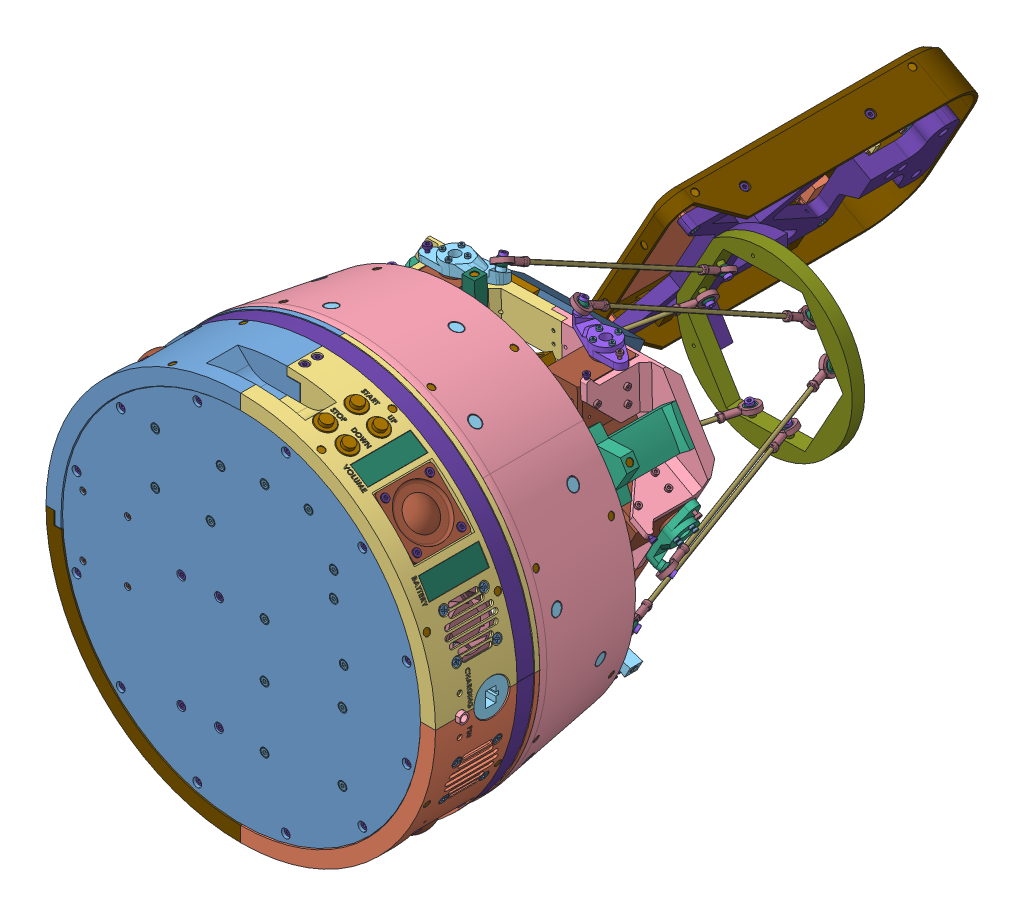
SolidWorks assembly robot xavier, configuration Défaut. Lengths in mm.
Overall size (438.41 438.41 602.06).
668 component instances, 95 part files, 20 mates.
Components (placement in the parent):
- base-1: base [Défaut] at (-67.3784 29.2661 438.4062) size (438.41 438.41 173)
  - base disk-1: base disk [Défaut] at (36.9194 20.0613 317) size (285 285 66.55)
    - base disk-1: base disk [Défaut] at (-39.9498 -9.3034 266.18) size (285 285 6.35)
    - Adafruit MAX9744-1: Adafruit MAX9744 [Défaut] at (-148.3839 -9.3034 256.18) x (0 1 0) z (0 0 -1) size (56.74 43.64 13.6)
    - Adafruit MAX9744-2: Adafruit MAX9744 [Défaut] at (-148.3839 -9.3034 239.58) x (0 1 0) z (0 0 -1) size (56.74 43.64 13.6)
    - Battery charger RRC-PMM240-1: Battery charger RRC-PMM240 [Défaut] at (-52.8471 67.1868 256.18) x (0 -1 0) z (0 0 -1) size (57 70 12)
    - battery holder-1: battery holder [Défaut] at (-92.9498 0.6966 266.18) x (0 -1 0) z (1 0 0) size (115 36.2 40)
    - Battery RRC2054-2-1: Battery RRC2054-2 [Défaut] at (-82.3791 -10.7125 233.18) x (0 1 0) z (0 0 1) size (151 78 23)
    - ground loop noise isolator-1: ground loop noise isolator [Défaut] at (-105.1098 -100.3034 233.18) x (0 -1 0) z (1 0 0) size (20 20 60)
    - ground loop noise isolator-2: ground loop noise isolator [Défaut] at (-45.1098 -80.3034 233.18) x (0 0 1) z (-1 0 0) size (20 20 60)
    - psu control-1: psu control [Défaut] at (-25.1498 95.1966 256.18) x (0 -1 0) z (0 0 -1) size (100 70 16.5)
    - buck boost-1: buck boost [Défaut] at (-25.6498 -27.3034 256.18) x (0 -1 0) z (0 0 -1) size (80 70 23.6)
    - buck boost-2: buck boost [Défaut] at (-25.6498 -27.3034 229.58) x (0 -1 0) z (0 0 -1) size (80 70 23.6)
    - 732-12936-ND-1: 732-12936-ND [Défaut] at (-166.1639 14.8266 254.58) x (-0.923728 -0.383049 0) z (0 0 -1) size (4.6 4.17 20)
    - 732-12936-ND-2: 732-12936-ND [Défaut] at (-166.1639 -33.4334 254.58) x (-0.923728 -0.383049 0) z (0 0 -1) size (4.6 4.17 20)
    - 732-12936-ND-3: 732-12936-ND [Défaut] at (-130.6039 -33.4334 254.58) x (-0.923728 -0.383049 0) z (0 0 -1) size (4.6 4.17 20)
    - 732-12936-ND-4: 732-12936-ND [Défaut] at (-130.6039 14.8266 254.58) x (-0.923728 -0.383049 0) z (0 0 -1) size (4.6 4.17 20)
    - 732-12918-ND-1: 732-12918-ND [Défaut] at (-166.1639 14.8266 266.18) x (-0.923728 -0.383049 0) z (0 0 -1) size (4.6 4.17 15)
    - 732-12918-ND-2: 732-12918-ND [Défaut] at (-130.6039 14.8266 266.18) x (-0.923728 -0.383049 0) z (0 0 -1) size (4.6 4.17 15)
    - 732-12918-ND-3: 732-12918-ND [Défaut] at (-130.6039 -33.4334 266.18) x (-0.923728 -0.383049 0) z (0 0 -1) size (4.6 4.17 15)
    - 732-12918-ND-4: 732-12918-ND [Défaut] at (-166.1639 -33.4334 266.18) x (-0.923728 -0.383049 0) z (0 0 -1) size (4.6 4.17 15)
    - M2x8mm socket-6: M2x8mm socket [Défaut] at (-166.1639 -33.4334 262.03) x (-1 0 0) z (0 0 1) size (3.8 3.8 9.6)
    - M2x8mm socket-5: M2x8mm socket [Défaut] at (-130.6039 -33.4334 262.03) x (-1 0 0) z (0 0 1) size (3.8 3.8 9.6)
    - M2x8mm socket-3: M2x8mm socket [Défaut] at (-166.1639 14.8266 262.03) size (3.8 3.8 9.6)
    - M2x8mm socket-4: M2x8mm socket [Défaut] at (-130.6039 14.8266 262.03) x (-1 0 0) z (0 0 1) size (3.8 3.8 9.6)
    - M2 nut-1: M2 nut [Défaut] at (-166.1639 14.8266 237.98) x (-0.923728 -0.383049 0) z (0 0 -1) size (4.62 4 1.6)
    - M2 nut-2: M2 nut [Défaut] at (-166.1639 -33.4334 237.98) x (-0.923728 -0.383049 0) z (0 0 -1) size (4.62 4 1.6)
    - M2 nut-3: M2 nut [Défaut] at (-130.6039 -33.4334 237.98) x (-0.923728 -0.383049 0) z (0 0 -1) size (4.62 4 1.6)
    - M2 nut-4: M2 nut [Défaut] at (-130.6039 14.8266 237.98) x (-0.923728 -0.383049 0) z (0 0 -1) size (4.62 4 1.6)
    - 36-24337-ND-1: 36-24337-ND [Défaut] at (-108.6498 86.6966 266.18) x (-0.923728 -0.383049 0) z (0 0 -1) size (5.77 5 18)
    - 36-24337-ND-2: 36-24337-ND [Défaut] at (-108.6498 45.6966 266.18) x (-0.923728 -0.383049 0) z (0 0 -1) size (5.77 5 18)
    - 36-24337-ND-3: 36-24337-ND [Défaut] at (-64.6498 44.6966 266.18) x (-0.923728 -0.383049 0) z (0 0 -1) size (5.77 5 18)
    - 36-24337-ND-4: 36-24337-ND [Défaut] at (-56.6498 86.6966 266.18) x (-0.923728 -0.383049 0) z (0 0 -1) size (5.77 5 18)
    - M3x5mm socket-1: M3x5mm socket [Défaut] at (-108.6498 86.6966 264.53) x (-1 0 0) z (0 0 1) size (5.5 5.5 8)
    - M3x5mm socket-2: M3x5mm socket [Défaut] at (-108.6498 45.6966 264.53) x (-1 0 0) z (0 0 1) size (5.5 5.5 8)
    - M3x5mm socket-3: M3x5mm socket [Défaut] at (-64.6498 44.6966 264.53) x (-1 0 0) z (0 0 1) size (5.5 5.5 8)
    - M3x5mm socket-4: M3x5mm socket [Défaut] at (-56.6498 86.6966 264.53) x (-1 0 0) z (0 0 1) size (5.5 5.5 8)
    - M3 nut-1: M3 nut [Défaut] at (-108.6498 86.6966 254.18) x (-0.923728 -0.383049 0) z (0 0 -1) size (6.35 5.5 2.4)
    - M3 nut-2: M3 nut [Défaut] at (-108.6498 45.6966 254.18) x (-0.923728 -0.383049 0) z (0 0 -1) size (6.35 5.5 2.4)
    - M3 nut-3: M3 nut [Défaut] at (-64.6498 44.6966 254.18) x (-0.923728 -0.383049 0) z (0 0 -1) size (6.35 5.5 2.4)
    - M3 nut-4: M3 nut [Défaut] at (-56.6498 86.6966 254.18) x (-0.923728 -0.383049 0) z (0 0 -1) size (6.35 5.5 2.4)
    - 36-24337-ND-5: 36-24337-ND [Défaut] at (-21.6498 91.6966 266.18) x (-0.923728 -0.383049 0) z (0 0 -1) size (5.77 5 18)
    - 36-24337-ND-6: 36-24337-ND [Défaut] at (-21.6498 -1.3034 266.18) x (1 0 0) z (0 0 -1) size (5.77 5 18)
    - 36-24337-ND-7: 36-24337-ND [Défaut] at (13.3502 91.6966 266.18) x (0.923728 0.383049 0) z (0 0 -1) size (5.77 5 18)
    - 36-24337-ND-8: 36-24337-ND [Défaut] at (41.3502 -1.3034 266.18) x (-1 0 0) z (0 0 -1) size (5.77 5 18)
    - M3 nut-5: M3 nut [Défaut] at (-21.6498 91.6966 256.98) x (-1 0 0) z (0 0 -1) size (6.35 5.5 2.4)
    - M3 nut-6: M3 nut [Défaut] at (13.3502 91.6966 252.18) x (-1 0 0) z (0 0 1) size (6.35 5.5 2.4)
    - M3 nut-7: M3 nut [Défaut] at (-21.6498 -1.3034 252.18) x (-1 0 0) z (0 0 1) size (6.35 5.5 2.4)
    - M3 nut-8: M3 nut [Défaut] at (41.3502 -1.3034 252.18) size (6.35 5.5 2.4)
    - 36-24337-ND-9: 36-24337-ND [Défaut] at (-21.6498 -44.3034 266.18) x (-0.923728 -0.383049 0) z (0 0 -1) size (5.77 5 18)
    - 36-24337-ND-10: 36-24337-ND [Défaut] at (-21.6498 -93.3034 266.18) x (-0.923728 -0.383049 0) z (0 0 -1) size (5.77 5 18)
    - 36-24337-ND-11: 36-24337-ND [Défaut] at (40.3502 -85.3034 266.18) x (-0.923728 -0.383049 0) z (0 0 -1) size (5.77 5 18)
    - 36-24337-ND-12: 36-24337-ND [Défaut] at (40.3502 -31.3034 266.18) x (-0.923728 -0.383049 0) z (0 0 -1) size (5.77 5 18)
    - 36-24342-ND-1: 36-24342-ND [Défaut] at (-21.6498 -44.3034 254.58) x (1 0 0) z (0 0 -1) size (5.77 5 33)
    - 36-24342-ND-2: 36-24342-ND [Défaut] at (-21.6498 -93.3034 254.58) x (1 0 0) z (0 0 -1) size (5.77 5 33)
    - 36-24342-ND-3: 36-24342-ND [Défaut] at (40.3502 -31.3034 254.58) x (1 0 0) z (0 0 -1) size (5.77 5 33)
    - 36-24342-ND-4: 36-24342-ND [Défaut] at (40.3502 -85.3034 254.58) x (1 0 0) z (0 0 -1) size (5.77 5 33)
    - M3 nut-9: M3 nut [Défaut] at (40.3502 -31.3034 227.98) x (-1 0 0) z (0 0 -1) size (6.35 5.5 2.4)
    - M3 nut-10: M3 nut [Défaut] at (-21.6498 -44.3034 227.98) x (-1 0 0) z (0 0 -1) size (6.35 5.5 2.4)
    - M3 nut-11: M3 nut [Défaut] at (-21.6498 -93.3034 225.58) size (6.35 5.5 2.4)
    - M3 nut-12: M3 nut [Défaut] at (40.3502 -85.3034 227.98) x (-1 0 0) z (0 0 -1) size (6.35 5.5 2.4)
    - 36-24337-ND-13: 36-24337-ND [Défaut] at (33.3502 60.1966 266.18) x (-0.923728 -0.383049 0) z (0 0 -1) size (5.77 5 18)
    - 36-24337-ND-14: 36-24337-ND [Défaut] at (33.3502 40.1966 266.18) x (-0.923728 -0.383049 0) z (0 0 -1) size (5.77 5 18)
    - M3 nut-13: M3 nut [Défaut] at (33.3502 60.1966 252.18) size (6.35 5.5 2.4)
    - M3 nut-14: M3 nut [Défaut] at (33.3502 40.1966 252.18) size (6.35 5.5 2.4)
    - M3x8mm plastic-1: M3x8mm plastic [Défaut] at (-57.9498 -4.3034 261.53) size (5.5 5.5 10.3)
    - M3x8mm plastic-2: M3x8mm plastic [Défaut] at (-57.9498 -94.3034 261.53) size (5.5 5.5 10.3)
    - M3x8mm plastic-3: M3x8mm plastic [Défaut] at (-87.9498 -94.3034 261.53) size (5.5 5.5 10.3)
    - M3x8mm plastic-4: M3x8mm plastic [Défaut] at (-87.9498 -4.3034 261.53) size (5.5 5.5 10.3)
    - M3x5mm socket-5: M3x5mm socket [Défaut] at (-21.6498 91.6966 264.53) size (5.5 5.5 8)
    - M3x5mm socket-6: M3x5mm socket [Défaut] at (13.3502 91.6966 264.53) size (5.5 5.5 8)
    - M3x5mm socket-7: M3x5mm socket [Défaut] at (33.3502 60.1966 264.53) size (5.5 5.5 8)
    - M3x5mm socket-8: M3x5mm socket [Défaut] at (33.3502 40.1966 264.53) size (5.5 5.5 8)
    - M3x5mm socket-9: M3x5mm socket [Défaut] at (-21.6498 -1.3034 264.53) size (5.5 5.5 8)
    - M3x5mm socket-10: M3x5mm socket [Défaut] at (-21.6498 -44.3034 264.53) size (5.5 5.5 8)
    - M3x5mm socket-11: M3x5mm socket [Défaut] at (-21.6498 -93.3034 264.53) size (5.5 5.5 8)
    - M3x5mm socket-12: M3x5mm socket [Défaut] at (40.3502 -85.3034 264.53) size (5.5 5.5 8)
    - M3x5mm socket-13: M3x5mm socket [Défaut] at (40.3502 -31.3034 264.53) size (5.5 5.5 8)
    - M3x5mm socket-14: M3x5mm socket [Défaut] at (41.3502 -1.3034 264.53) size (5.5 5.5 8)
  - base audio-1: base audio [Défaut] at (-77.1238 -92.9542 353.528) x (0 1 0) z (0 0 1) size (420.86 420.86 86)
    - base audio front left-1: base audio front left [Défaut] at (103.7122 -74.0934 171.652) size (155 165 86)
    - base audio front right-1: base audio front right [Défaut] at (103.7122 -74.0934 171.652) x (0 -1 0) z (0 0 1) size (165 165 86)
    - base audio back left-1: base audio back left [Défaut] at (103.7122 -74.0934 171.652) x (0 1 0) z (0 0 1) size (155 156 86)
    - base audio back right-1: base audio back right [Défaut] at (103.7122 -74.0934 171.652) x (-1 0 0) z (0 0 1) size (156 155 86)
    - SC2073-ND-1: SC2073-ND [Défaut] at (103.7122 -222.6934 217.152) x (1 0 0) z (0 -1 0) size (11.94 11.94 36.36)
    - RJ45 connector-1: RJ45 connector [Défaut] at (103.7122 -228.0934 191.652) x (1 0 0) z (0 1 0) size (27.9 27.9 35.9)
    - Micro USB B (Adafruit 4217)-1: Micro USB B (Adafruit 4217) [Défaut] at (-6.0335 -126.2291 211.652) x (-0.429101 0.903257 0) z (0 0 1) size (28 33.5 28)
    - Micro USB B nut (Adafruit 4217)-1: Micro USB B nut (Adafruit 4217) [Défaut] at (-28.6149 -136.9566 211.652) x (0.18262 -0.384415 -0.904917) z (0.903257 0.429101 0) size (30.02 30.02 8)
    - switch-1: switch [Défaut] at (-36.2542 -140.9179 186.027) x (0.429101 -0.903257 0) z (0.903257 0.429101 0) size (20.75 14.7 24.67)
    - button-1: button [Défaut] at (254.7907 -122.0257 191.152) x (0.197389 0.622151 -0.757605) z (-0.953177 0.302412 0) size (14 14 27.8)
    - button-2: button [Défaut] at (247.8231 -140.0803 191.152) x (0.179537 0.392097 -0.902234) z (-0.909218 0.416321 0) size (14 14 27.8)
    - button-3: button [Défaut] at (254.7907 -122.0257 216.152) x (0.197389 0.622151 -0.757605) z (-0.953177 0.302412 0) size (14 14 27.8)
    - button-4: button [Défaut] at (247.8231 -140.0803 216.152) x (0.179537 0.392097 -0.902234) z (-0.909218 0.416321 0) size (14 14 27.8)
    - button nut-1: button nut [Défaut] at (247.1653 -119.6064 191.152) x (0.099317 0.313039 0.944533) z (-0.953177 0.302412 0) size (16 16 5)
    - button nut-2: button nut [Défaut] at (247.1653 -119.6064 216.152) x (0.099317 0.313039 0.944533) z (-0.953177 0.302412 0) size (16 16 5)
    - button nut-3: button nut [Défaut] at (240.5494 -136.7497 216.152) x (0.182325 0.398185 0.899003) z (-0.909218 0.416321 0) size (16 16 5)
    - button nut-4: button nut [Défaut] at (240.5494 -136.7497 191.152) x (0.179537 0.392097 -0.902234) z (-0.909218 0.416321 0) size (16 16 5) (hidden)
    - Dayton Audio DMA45-8-1: Dayton Audio DMA45-8 [Défaut] at (209.7782 -180.1594 199.652) x (0.707107 0.707107 0) z (0.707107 -0.707107 0) size (46 46 32.1)
    - Dayton Audio DMA45-8-2: Dayton Audio DMA45-8 [Défaut] at (209.7782 31.9727 199.652) x (-0.707107 0.707107 0) z (0.707107 0.707107 0) size (46 46 32.1)
    - Dayton Audio DMA45-8-3: Dayton Audio DMA45-8 [Défaut] at (-2.3539 31.9727 199.652) x (-0.707107 -0.707107 0) z (-0.707107 0.707107 0) size (46 46 32.1)
    - Dayton Audio DMA45-8-4: Dayton Audio DMA45-8 [Défaut] at (-2.3539 -180.1594 199.652) x (0.707107 -0.707107 0) z (-0.707107 -0.707107 0) size (46 46 32.1)
    - LED 5mm-1: LED 5mm [Défaut] at (88.5685 -227.8494 216.652) x (-0.876134 0.086292 -0.474281) z (0.098017 0.995185 0) size (5.5 5.5 18.7)
    - LED 5mm-2: LED 5mm [Défaut] at (118.8558 -227.8494 216.652) x (-0.780695 -0.076892 -0.620163) z (-0.098017 0.995185 0) size (5.5 5.5 18.7)
    - Noctua NF-A4X20-1: Noctua NF-A4X20 [Défaut] at (61.6633 -197.158 199.652) x (0.946287 -0.323328 0) z (-0.323328 -0.946287 0) size (39.9 39.9 19.95)
    - Noctua NF-A4X20-2: Noctua NF-A4X20 [Défaut] at (145.761 -197.158 199.652) x (0.946287 0.323328 0) z (0.323328 -0.946287 0) size (39.9 39.9 19.95)
    - LED level-1: LED level [Défaut] at (232.9084 -146.5387 181.6389) x (0.524024 0.851704 0) z (0.851704 -0.524024 0) size (12 34.5 2)
    - LED level-2: LED level [Défaut] at (185.0786 -197.8654 181.6389) x (0.857177 0.515023 0) z (0.515023 -0.857177 0) size (12 34.5 2)
    - LED level diffuser-1: LED level diffuser [Défaut] at (240.4553 -143.8142 199.2629) x (0.524024 0.851704 0) z (0.851704 -0.524024 0) size (16 47.5 1.59)
    - LED level diffuser-2: LED level diffuser [Défaut] at (193.0327 -198.9193 199.2629) x (0.857177 0.515023 0) z (0.515023 -0.857177 0) size (16 47.5 1.59)
    - LED strip-1: LED strip [Défaut] at (103.7122 -74.0934 159.902) x (0.707107 -0.707107 0) z (0 0 1) size (297.3 297.88 9.5)
    - LED strip diffuser (round)-1: LED strip diffuser (round) [Défaut] at (103.7122 -74.0934 157.902) x (0.000809 -1 0) z (0 0 1) size (309.17 309.17 13.5)
    - light sensor-1: light sensor [Défaut] at (228.5122 -87.4674 238.7403) x (0 0 -1) z (1 0 0) size (7.62 10.16 4.2)
    - light sensor-2: light sensor [Défaut] at (-21.0878 -87.4674 196.0637) x (0 0 1) z (-1 0 0) size (7.62 10.16 4.2)
    - light sensor-3: light sensor [Défaut] at (29.9331 -198.7828 198.0637) x (0 0 1) z (-0.537899 -0.843009 0) size (7.62 10.16 4.2)
    - light sensor-4: light sensor [Défaut] at (109.4763 70.6739 198.0637) x (0 0 1) z (0.073377 0.997304 0) size (7.62 10.16 4.2)
    - M3x8mm plastic-1: M3x8mm plastic [Défaut] at (98.7122 69.9066 183.652) x (1 0 0) z (0 1 0) size (5.5 5.5 10.3)
    - M3x8mm plastic-2: M3x8mm plastic [Défaut] at (98.7122 69.9066 213.652) x (1 0 0) z (0 1 0) size (5.5 5.5 10.3)
    - M3x8mm plastic-3: M3x8mm plastic [Défaut] at (-40.2878 -79.0934 180.652) x (0 0 1) z (-1 0 0) size (5.5 5.5 10.3)
    - M3x8mm plastic-4: M3x8mm plastic [Défaut] at (-40.2878 -79.0934 190.652) x (0 0 1) z (-1 0 0) size (5.5 5.5 10.3)
    - M3x8mm plastic-5: M3x8mm plastic [Défaut] at (247.7122 -79.0934 180.652) x (0 0 -1) z (1 0 0) size (5.5 5.5 10.3)
    - M3x8mm plastic-6: M3x8mm plastic [Défaut] at (247.7122 -79.0934 190.652) x (0 0 -1) z (1 0 0) size (5.5 5.5 10.3)
    - M3x8mm plastic-8: M3x8mm plastic [Défaut] at (192.6308 -188.1143 181.902) x (0.5 0.5 -0.707107) z (0.707107 -0.707107 0) size (5.5 5.5 10.3)
    - M3x8mm plastic-14: M3x8mm plastic [Défaut] at (-10.3088 -163.012 181.902) x (0.5 -0.5 -0.707107) z (-0.707107 -0.707107 0) size (5.5 5.5 10.3)
    - M3x8mm plastic-13: M3x8mm plastic [Défaut] at (14.7935 39.9276 181.902) x (-0.5 -0.5 -0.707107) z (-0.707107 0.707107 0) size (5.5 5.5 10.3)
    - M3x8mm plastic-12: M3x8mm plastic [Défaut] at (217.7331 14.8253 181.902) x (-0.5 0.5 -0.707107) z (0.707107 0.707107 0) size (5.5 5.5 10.3)
    - M3x8mm plastic-9: M3x8mm plastic [Défaut] at (217.7331 -163.012 217.402) x (0.5 0.5 -0.707107) z (0.707107 -0.707107 0) size (5.5 5.5 10.3)
    - M3x8mm plastic-17: M3x8mm plastic [Défaut] at (14.7935 -188.1143 217.402) x (0.5 -0.5 -0.707107) z (-0.707107 -0.707107 0) size (5.5 5.5 10.3)
    - M3x8mm plastic-16: M3x8mm plastic [Défaut] at (-10.3088 14.8253 217.402) x (-0.5 -0.5 -0.707107) z (-0.707107 0.707107 0) size (5.5 5.5 10.3)
    - M3x8mm plastic-15: M3x8mm plastic [Défaut] at (192.6308 39.9276 217.402) x (-0.5 0.5 -0.707107) z (0.707107 0.707107 0) size (5.5 5.5 10.3)
    - M3x8mm plastic-10: M3x8mm plastic [Défaut] at (192.6308 -188.1143 217.402) x (0.5 0.5 -0.707107) z (0.707107 -0.707107 0) size (5.5 5.5 10.3)
    - M3x8mm plastic-20: M3x8mm plastic [Défaut] at (-10.3088 -163.012 217.402) x (0.5 -0.5 -0.707107) z (-0.707107 -0.707107 0) size (5.5 5.5 10.3)
    - M3x8mm plastic-19: M3x8mm plastic [Défaut] at (14.7935 39.9276 217.402) x (-0.5 -0.5 -0.707107) z (-0.707107 0.707107 0) size (5.5 5.5 10.3)
    - M3x8mm plastic-18: M3x8mm plastic [Défaut] at (217.7331 14.8253 217.402) x (-0.5 0.5 -0.707107) z (0.707107 0.707107 0) size (5.5 5.5 10.3)
    - M3x8mm plastic-11: M3x8mm plastic [Défaut] at (217.7331 -163.012 181.902) x (0.5 0.5 -0.707107) z (0.707107 -0.707107 0) size (5.5 5.5 10.3)
    - M3x8mm plastic-23: M3x8mm plastic [Défaut] at (14.7935 -188.1143 181.902) x (0.5 -0.5 -0.707107) z (-0.707107 -0.707107 0) size (5.5 5.5 10.3)
    - M3x8mm plastic-22: M3x8mm plastic [Défaut] at (-10.3088 14.8253 181.902) x (-0.5 -0.5 -0.707107) z (-0.707107 0.707107 0) size (5.5 5.5 10.3)
    - M3x8mm plastic-21: M3x8mm plastic [Défaut] at (192.6308 39.9276 181.902) x (-0.5 0.5 -0.707107) z (0.707107 0.707107 0) size (5.5 5.5 10.3)
    - fan screw-1: fan screw [Défaut] at (165.5737 -205.6586 183.652) x (0.879667 0.300565 -0.368573) z (0.323328 -0.946287 0) size (6.3 6.3 9.5)
    - fan screw-2: fan screw [Défaut] at (165.5737 -205.6586 215.652) x (0.879667 0.300565 -0.368573) z (0.323328 -0.946287 0) size (6.3 6.3 9.5)
    - fan screw-3: fan screw [Défaut] at (135.2925 -216.0051 215.652) x (-0.927498 -0.316908 -0.198283) z (0.323328 -0.946287 0) size (6.3 6.3 9.5)
    - fan screw-4: fan screw [Défaut] at (135.2925 -216.0051 183.652) x (0.879667 0.300565 -0.368573) z (0.323328 -0.946287 0) size (6.3 6.3 9.5)
    - fan screw-5: fan screw [Défaut] at (72.1318 -216.0051 183.652) x (0.879667 -0.300565 0.368573) z (-0.323328 -0.946287 0) size (6.3 6.3 9.5)
    - fan screw-6: fan screw [Défaut] at (72.1318 -216.0051 215.652) x (0.879667 -0.300565 0.368573) z (-0.323328 -0.946287 0) size (6.3 6.3 9.5)
    - fan screw-7: fan screw [Défaut] at (41.8506 -205.6586 215.652) x (0.879667 -0.300565 0.368573) z (-0.323328 -0.946287 0) size (6.3 6.3 9.5)
    - fan screw-8: fan screw [Défaut] at (41.8506 -205.6586 183.652) x (0.879667 -0.300565 0.368573) z (-0.323328 -0.946287 0) size (6.3 6.3 9.5)
    - dewel pin 0.125in 0.5in-1: dewel pin 0.125in 0.5in [Défaut] at (111.2122 -212.8434 155.652) x (0 0 1) z (-1 0 0) size (3.17 3.17 12.7)
    - dewel pin 0.125in 0.5in-2: dewel pin 0.125in 0.5in [Défaut] at (111.2122 -223.0934 228.6844) x (0 0 1) z (-1 0 0) size (3.17 3.17 12.7)
    - M2x5mm plastic-1: M2x5mm plastic [Défaut] at (233.5122 -79.5934 217.402) x (0 0.924225 0.381849) z (-1 0 0) size (3.35 3.35 6.6)
    - M2x5mm plastic-2: M2x5mm plastic [Défaut] at (-26.0878 -79.5934 217.402) x (0 0.5 -0.866025) z (1 0 0) size (3.35 3.35 6.6)
    - M2x5mm plastic-3: M2x5mm plastic [Défaut] at (20.6058 -198.7624 219.402) x (-0.826053 0.527081 -0.199554) z (0.537899 0.843009 0) size (3.35 3.35 6.6)
    - M2x5mm plastic-4: M2x5mm plastic [Défaut] at (117.696 75.0827 219.402) x (0.994616 -0.073179 0.073377) z (-0.073377 -0.997304 0) size (3.35 3.35 6.6)
  - base mic-1: base mic [Défaut] at (-78.91 184.7021 463.131) x (-0.707107 -0.707107 0) z (0.707107 -0.707107 0) size (310 92.85 310)
    - base mic-1: base mic [Défaut] at (69.3421 -41.049 176.652) size (155 90 160)
    - 8SoundsUSB Mic-1: 8SoundsUSB Mic [Défaut] at (30.5719 -34.8926 320.3049) x (0.980785 0 0.19509) z (-0.192688 0.156434 0.96871) size (25.4 23.4 21.48)
    - 8SoundsUSB Mic-2: 8SoundsUSB Mic [Défaut] at (-17.8103 6.4759 289.0854) x (0.83147 0 0.55557) z (-0.54873 0.156434 0.821233) size (25.4 23.4 21.48)
    - 8SoundsUSB Mic-3: 8SoundsUSB Mic [Défaut] at (-71.7864 6.4759 194.5283) x (0.19509 0 0.980785) z (-0.96871 0.156434 0.192688) size (25.4 23.4 21.48)
    - 8SoundsUSB Mic-4: 8SoundsUSB Mic [Défaut] at (-59.6505 -34.8926 250.8153) x (0.55557 0 0.83147) z (-0.821233 0.156434 0.54873) size (25.4 23.4 21.48)
    - 16SoundsUSB-1: 16SoundsUSB [Défaut] at (69.3421 -36.049 176.6521) x (1 0 0) z (0 -1 0) size (165.86 165.78 26.13)
    - M3x5mm plastic-1: M3x5mm plastic [Défaut] at (49.8528 -16.3964 325.89) x (-0.186611 0.963352 -0.192688) z (0.192688 -0.156434 -0.96871) size (5.5 5.5 7.3)
    - M3x5mm plastic-2: M3x5mm plastic [Défaut] at (30.2371 -16.3964 321.9882) x (-0.186611 0.963352 -0.192688) z (0.192688 -0.156434 -0.96871) size (5.5 5.5 7.3)
    - M3x5mm plastic-3: M3x5mm plastic [Défaut] at (49.3034 -34.1748 328.6517) x (-0.186611 0.963352 -0.192688) z (0.192688 -0.156434 -0.96871) size (5.5 5.5 7.3)
    - M3x5mm plastic-4: M3x5mm plastic [Défaut] at (29.6877 -34.1748 324.7499) x (-0.186611 0.963352 -0.192688) z (0.192688 -0.156434 -0.96871) size (5.5 5.5 7.3)
    - M3x5mm plastic-5: M3x5mm plastic [Défaut] at (-2.1344 24.9721 301.6238) x (-0.684341 0.480179 -0.54873) z (0.54873 -0.156434 -0.821233) size (5.5 5.5 7.3)
    - M3x5mm plastic-6: M3x5mm plastic [Défaut] at (-18.7638 24.9721 290.5124) x (-0.684341 0.480179 -0.54873) z (0.54873 -0.156434 -0.821233) size (5.5 5.5 7.3)
    - M3x5mm plastic-7: M3x5mm plastic [Défaut] at (-3.6988 7.1937 303.965) x (-0.684341 0.480179 -0.54873) z (0.54873 -0.156434 -0.821233) size (5.5 5.5 7.3)
    - M3x5mm plastic-8: M3x5mm plastic [Défaut] at (-20.3282 7.1937 292.8536) x (-0.684341 0.480179 -0.54873) z (0.54873 -0.156434 -0.821233) size (5.5 5.5 7.3)
    - M3x5mm plastic-9: M3x5mm plastic [Défaut] at (-49.9661 -16.3964 268.3981) x (-0.494502 0.284684 -0.821233) z (0.821233 -0.156434 -0.54873) size (5.5 5.5 7.3)
    - M3x5mm plastic-10: M3x5mm plastic [Défaut] at (-61.0775 -16.3964 251.7687) x (-0.494502 0.284684 -0.821233) z (0.821233 -0.156434 -0.54873) size (5.5 5.5 7.3)
    - M3x5mm plastic-11: M3x5mm plastic [Défaut] at (-63.4188 -34.1748 253.3331) x (-0.494502 0.284684 -0.821233) z (0.821233 -0.156434 -0.54873) size (5.5 5.5 7.3)
    - M3x5mm plastic-12: M3x5mm plastic [Défaut] at (-52.3074 -34.1748 269.9625) x (-0.494502 0.284684 -0.821233) z (0.821233 -0.156434 -0.54873) size (5.5 5.5 7.3)
    - M3x5mm plastic-13: M3x5mm plastic [Défaut] at (-72.3295 7.1937 215.0282) x (-0.225994 -0.876896 -0.424241) z (0.96871 -0.156434 -0.192688) size (5.5 5.5 7.3)
    - M3x5mm plastic-14: M3x5mm plastic [Défaut] at (-69.5678 24.9721 214.4788) x (-0.162376 0.187709 -0.96871) z (0.96871 -0.156434 -0.192688) size (5.5 5.5 7.3)
    - M3x5mm plastic-15: M3x5mm plastic [Défaut] at (-73.4696 24.9721 194.8631) x (-0.162376 0.187709 -0.96871) z (0.96871 -0.156434 -0.192688) size (5.5 5.5 7.3)
    - M3x5mm plastic-16: M3x5mm plastic [Défaut] at (-76.2313 7.1937 195.4125) x (-0.162376 0.187709 -0.96871) z (0.96871 -0.156434 -0.192688) size (5.5 5.5 7.3)
    - M3x8mm plastic-1: M3x8mm plastic [Défaut] at (15.9671 -42.4056 230.027) x (1 0 0) z (0 1 0) size (5.5 5.5 10.3)
    - M3x8mm plastic-2: M3x8mm plastic [Défaut] at (122.7171 -42.4056 230.027) x (1 0 0) z (0 1 0) size (5.5 5.5 10.3)
    - M3x8mm plastic-3: M3x8mm plastic [Défaut] at (15.9671 -42.4056 123.277) x (-0.837169 0 -0.546944) z (0 1 0) size (5.5 5.5 10.3)
    - M3x8mm plastic-4: M3x8mm plastic [Défaut] at (122.7171 -42.4056 123.277) x (-0.837169 0 -0.546944) z (0 1 0) size (5.5 5.5 10.3)
    - M3x5mm plastic-17: M3x5mm plastic [Défaut] at (-75.994 -16.3964 137.547) x (0.192688 0.963352 -0.186611) z (0.96871 -0.156434 0.192688) size (5.5 5.5 7.3)
    - M3x5mm plastic-18: M3x5mm plastic [Défaut] at (108.4472 -16.3964 31.3159) x (0.186611 0.963352 0.192688) z (-0.192688 -0.156434 0.96871) size (5.5 5.5 7.3)
    - M3x5mm plastic-19: M3x5mm plastic [Défaut] at (214.6783 -16.3964 215.7571) x (-0.192688 0.963352 0.186611) z (-0.96871 -0.156434 -0.192688) size (5.5 5.5 7.3)
    - M3x5mm plastic-20: M3x5mm plastic [Défaut] at (-82.6575 -34.1748 156.6133) x (0.192688 0.963352 -0.186611) z (0.96871 -0.156434 0.192688) size (5.5 5.5 7.3)
    - M3x5mm plastic-21: M3x5mm plastic [Défaut] at (89.3808 -34.1748 24.6524) x (0.186611 0.963352 0.192688) z (-0.192688 -0.156434 0.96871) size (5.5 5.5 7.3)
    - M3x5mm plastic-22: M3x5mm plastic [Défaut] at (221.3418 -34.1748 196.6907) x (-0.192688 0.963352 0.186611) z (-0.96871 -0.156434 -0.192688) size (5.5 5.5 7.3)
    - M3x5mm plastic-23: M3x5mm plastic [Défaut] at (-78.7557 -34.1748 136.9976) x (0.192688 0.963352 -0.186611) z (0.96871 -0.156434 0.192688) size (5.5 5.5 7.3)
    - M3x5mm plastic-24: M3x5mm plastic [Défaut] at (108.9965 -34.1748 28.5542) x (0.186611 0.963352 0.192688) z (-0.192688 -0.156434 0.96871) size (5.5 5.5 7.3)
    - M3x5mm plastic-25: M3x5mm plastic [Défaut] at (217.44 -34.1748 216.3064) x (-0.192688 0.963352 0.186611) z (-0.96871 -0.156434 -0.192688) size (5.5 5.5 7.3)
    - M3x5mm plastic-26: M3x5mm plastic [Défaut] at (-55.6296 24.9721 105.1755) x (0.54873 0.480179 -0.684341) z (0.821233 -0.156434 0.54873) size (5.5 5.5 7.3)
    - M3x5mm plastic-27: M3x5mm plastic [Défaut] at (140.8187 24.9721 51.6803) x (0.684341 0.480179 0.54873) z (-0.54873 -0.156434 0.821233) size (5.5 5.5 7.3)
    - M3x5mm plastic-28: M3x5mm plastic [Défaut] at (194.3139 24.9721 248.1286) x (-0.54873 0.480179 0.684341) z (-0.821233 -0.156434 -0.54873) size (5.5 5.5 7.3)
    - M3x5mm plastic-29: M3x5mm plastic [Défaut] at (-44.5182 24.9721 88.5461) x (0.54873 0.480179 -0.684341) z (0.821233 -0.156434 0.54873) size (5.5 5.5 7.3)
    - M3x5mm plastic-30: M3x5mm plastic [Défaut] at (157.4481 24.9721 62.7917) x (0.684341 0.480179 0.54873) z (-0.54873 -0.156434 0.821233) size (5.5 5.5 7.3)
    - M3x5mm plastic-31: M3x5mm plastic [Défaut] at (183.2025 24.9721 264.758) x (-0.54873 0.480179 0.684341) z (-0.821233 -0.156434 -0.54873) size (5.5 5.5 7.3)
    - M3x5mm plastic-32: M3x5mm plastic [Défaut] at (-57.9709 7.1937 103.6111) x (0.54873 0.480179 -0.684341) z (0.821233 -0.156434 0.54873) size (5.5 5.5 7.3)
    - M3x5mm plastic-33: M3x5mm plastic [Défaut] at (142.3831 7.1937 49.339) x (0.684341 0.480179 0.54873) z (-0.54873 -0.156434 0.821233) size (5.5 5.5 7.3)
    - M3x5mm plastic-34: M3x5mm plastic [Défaut] at (196.6551 7.1937 249.693) x (-0.54873 0.480179 0.684341) z (-0.821233 -0.156434 -0.54873) size (5.5 5.5 7.3)
    - M3x5mm plastic-35: M3x5mm plastic [Défaut] at (-46.8595 7.1937 86.9817) x (0.54873 0.480179 -0.684341) z (0.821233 -0.156434 0.54873) size (5.5 5.5 7.3)
    - M3x5mm plastic-36: M3x5mm plastic [Défaut] at (159.0125 7.1937 60.4504) x (0.684341 0.480179 0.54873) z (-0.54873 -0.156434 0.821233) size (5.5 5.5 7.3)
    - M3x5mm plastic-37: M3x5mm plastic [Défaut] at (185.5437 7.1937 266.3224) x (-0.54873 0.480179 0.684341) z (-0.821233 -0.156434 -0.54873) size (5.5 5.5 7.3)
    - M3x5mm plastic-38: M3x5mm plastic [Défaut] at (-22.404 -16.3964 57.3438) x (0.821233 0.284684 -0.494502) z (0.54873 -0.156434 0.821233) size (5.5 5.5 7.3)
    - M3x5mm plastic-39: M3x5mm plastic [Défaut] at (188.6504 -16.3964 84.9059) x (0.494502 0.284684 0.821233) z (-0.821233 -0.156434 0.54873) size (5.5 5.5 7.3)
    - M3x5mm plastic-40: M3x5mm plastic [Défaut] at (161.0882 -16.3964 295.9603) x (-0.821233 0.284684 0.494502) z (-0.54873 -0.156434 -0.821233) size (5.5 5.5 7.3)
    - M3x5mm plastic-41: M3x5mm plastic [Défaut] at (-5.7746 -16.3964 46.2324) x (0.821233 0.284684 -0.494502) z (0.54873 -0.156434 0.821233) size (5.5 5.5 7.3)
    - M3x5mm plastic-42: M3x5mm plastic [Défaut] at (199.7618 -16.3964 101.5353) x (0.494502 0.284684 0.821233) z (-0.821233 -0.156434 0.54873) size (5.5 5.5 7.3)
    - M3x5mm plastic-43: M3x5mm plastic [Défaut] at (144.4588 -16.3964 307.0717) x (-0.821233 0.284684 0.494502) z (-0.54873 -0.156434 -0.821233) size (5.5 5.5 7.3)
    - M3x5mm plastic-44: M3x5mm plastic [Défaut] at (-7.339 -34.1748 43.8911) x (0.821233 0.284684 -0.494502) z (0.54873 -0.156434 0.821233) size (5.5 5.5 7.3)
    - M3x5mm plastic-45: M3x5mm plastic [Défaut] at (202.103 -34.1748 99.9709) x (0.494502 0.284684 0.821233) z (-0.821233 -0.156434 0.54873) size (5.5 5.5 7.3)
    - M3x5mm plastic-46: M3x5mm plastic [Défaut] at (146.0232 -34.1748 309.4129) x (-0.821233 0.284684 0.494502) z (-0.54873 -0.156434 -0.821233) size (5.5 5.5 7.3)
    - M3x5mm plastic-47: M3x5mm plastic [Défaut] at (-23.9684 -34.1748 55.0025) x (0.821233 0.284684 -0.494502) z (0.54873 -0.156434 0.821233) size (5.5 5.5 7.3)
    - M3x5mm plastic-48: M3x5mm plastic [Défaut] at (190.9916 -34.1748 83.3415) x (0.494502 0.284684 0.821233) z (-0.821233 -0.156434 0.54873) size (5.5 5.5 7.3)
    - M3x5mm plastic-49: M3x5mm plastic [Défaut] at (162.6526 -34.1748 298.3015) x (-0.821233 0.284684 0.494502) z (-0.54873 -0.156434 -0.821233) size (5.5 5.5 7.3)
    - M3x5mm plastic-50: M3x5mm plastic [Défaut] at (30.966 7.1937 34.9804) x (0.424241 -0.876896 -0.225994) z (0.192688 -0.156434 0.96871) size (5.5 5.5 7.3)
    - M3x5mm plastic-51: M3x5mm plastic [Défaut] at (211.0138 7.1937 138.2759) x (0.225994 -0.876896 0.424241) z (-0.96871 -0.156434 0.192688) size (5.5 5.5 7.3)
    - M3x5mm plastic-52: M3x5mm plastic [Défaut] at (107.7183 7.1937 318.3237) x (-0.424241 -0.876896 0.225994) z (-0.192688 -0.156434 -0.96871) size (5.5 5.5 7.3)
    - M3x5mm plastic-53: M3x5mm plastic [Défaut] at (31.5153 24.9721 37.7421) x (0.96871 0.187709 -0.162376) z (0.192688 -0.156434 0.96871) size (5.5 5.5 7.3)
    - M3x5mm plastic-54: M3x5mm plastic [Défaut] at (208.252 24.9721 138.8252) x (0.162376 0.187709 0.96871) z (-0.96871 -0.156434 0.192688) size (5.5 5.5 7.3)
    - M3x5mm plastic-55: M3x5mm plastic [Défaut] at (107.1689 24.9721 315.5619) x (-0.96871 0.187709 0.162376) z (-0.192688 -0.156434 -0.96871) size (5.5 5.5 7.3)
    - M3x5mm plastic-56: M3x5mm plastic [Défaut] at (51.131 24.9721 33.8403) x (0.96871 0.187709 -0.162376) z (0.192688 -0.156434 0.96871) size (5.5 5.5 7.3)
    - M3x5mm plastic-57: M3x5mm plastic [Défaut] at (212.1539 24.9721 158.4409) x (0.162376 0.187709 0.96871) z (-0.96871 -0.156434 0.192688) size (5.5 5.5 7.3)
    - M3x5mm plastic-58: M3x5mm plastic [Défaut] at (87.5532 24.9721 319.4638) x (-0.96871 0.187709 0.162376) z (-0.192688 -0.156434 -0.96871) size (5.5 5.5 7.3)
    - M3x5mm plastic-59: M3x5mm plastic [Défaut] at (50.5817 7.1937 31.0786) x (0.96871 0.187709 -0.162376) z (0.192688 -0.156434 0.96871) size (5.5 5.5 7.3)
    - M3x5mm plastic-60: M3x5mm plastic [Défaut] at (214.9156 7.1937 157.8916) x (0.162376 0.187709 0.96871) z (-0.96871 -0.156434 0.192688) size (5.5 5.5 7.3)
    - M3x5mm plastic-61: M3x5mm plastic [Défaut] at (88.1026 7.1937 322.2255) x (-0.96871 0.187709 0.162376) z (-0.192688 -0.156434 -0.96871) size (5.5 5.5 7.3)
    - M3x5mm plastic-62: M3x5mm plastic [Défaut] at (-79.8958 -16.3964 157.1627) x (0.192688 0.963352 -0.186611) z (0.96871 -0.156434 0.192688) size (5.5 5.5 7.3)
    - M3x5mm plastic-63: M3x5mm plastic [Défaut] at (88.8315 -16.3964 27.4141) x (0.186611 0.963352 0.192688) z (-0.192688 -0.156434 0.96871) size (5.5 5.5 7.3)
    - M3x5mm plastic-64: M3x5mm plastic [Défaut] at (218.5801 -16.3964 196.1414) x (-0.192688 0.963352 0.186611) z (-0.96871 -0.156434 -0.192688) size (5.5 5.5 7.3)
    - 8SoundsUSB Mic-17: 8SoundsUSB Mic [Défaut] at (-4.8211 -34.8926 47.6594) x (-0.83147 0 0.55557) z (-0.54873 0.156434 -0.821233) size (25.4 23.4 21.48)
    - 8SoundsUSB Mic-18: 8SoundsUSB Mic [Défaut] at (198.3348 -34.8926 102.4888) x (-0.55557 0 -0.83147) z (0.821233 0.156434 -0.54873) size (25.4 23.4 21.48)
    - 8SoundsUSB Mic-19: 8SoundsUSB Mic [Défaut] at (143.5054 -34.8926 305.6447) x (0.83147 0 -0.55557) z (0.54873 0.156434 0.821233) size (25.4 23.4 21.48)
    - 8SoundsUSB Mic-20: 8SoundsUSB Mic [Défaut] at (51.4658 6.4759 35.5235) x (-0.980785 0 0.19509) z (-0.192688 0.156434 -0.96871) size (25.4 23.4 21.48)
    - 8SoundsUSB Mic-21: 8SoundsUSB Mic [Défaut] at (210.4706 6.4759 158.7758) x (-0.19509 0 -0.980785) z (0.96871 0.156434 -0.192688) size (25.4 23.4 21.48)
    - 8SoundsUSB Mic-22: 8SoundsUSB Mic [Défaut] at (87.2184 6.4759 317.7805) x (0.980785 0 -0.19509) z (0.192688 0.156434 0.96871) size (25.4 23.4 21.48)
    - 8SoundsUSB Mic-23: 8SoundsUSB Mic [Défaut] at (-43.0912 6.4759 89.4996) x (-0.55557 0 0.83147) z (-0.821233 0.156434 -0.54873) size (25.4 23.4 21.48)
    - 8SoundsUSB Mic-24: 8SoundsUSB Mic [Défaut] at (156.4946 6.4759 64.2187) x (-0.83147 0 -0.55557) z (0.54873 0.156434 -0.821233) size (25.4 23.4 21.48)
    - 8SoundsUSB Mic-25: 8SoundsUSB Mic [Défaut] at (181.7755 6.4759 263.8045) x (0.55557 0 -0.83147) z (0.821233 0.156434 0.54873) size (25.4 23.4 21.48)
    - 8SoundsUSB Mic-26: 8SoundsUSB Mic [Défaut] at (-74.3108 -34.8926 137.8818) x (-0.19509 0 0.980785) z (-0.96871 0.156434 -0.192688) size (25.4 23.4 21.48)
    - 8SoundsUSB Mic-27: 8SoundsUSB Mic [Défaut] at (108.1124 -34.8926 32.9991) x (-0.980785 0 -0.19509) z (0.192688 0.156434 -0.96871) size (25.4 23.4 21.48)
    - 8SoundsUSB Mic-28: 8SoundsUSB Mic [Défaut] at (212.995 -34.8926 215.4223) x (0.19509 0 -0.980785) z (0.96871 0.156434 0.192688) size (25.4 23.4 21.48)
    - base mic-5: base mic [Défaut] at (69.3421 -41.049 176.652) x (0 0 1) z (-1 0 0) size (155 90 160)
    - base mic-6: base mic [Défaut] at (69.3421 -41.049 176.652) x (-1 0 0) z (0 0 -1) size (155 90 160)
    - base mic-7: base mic [Défaut] at (69.3421 -41.049 176.652) x (0 0 -1) z (1 0 0) size (155 90 160)
  - M3x8mm plastic-1: M3x8mm plastic [Défaut] at (93.1361 106.9245 577.53) size (5.5 5.5 10.3)
  - M3x12mm plastic-1: M3x12mm plastic [Défaut] at (-55.8407 -116.7374 511.18) x (-0.923728 -0.383049 0) z (0 0 -1) size (5.5 5.5 14.3)
  - M3x8mm plastic-13: M3x8mm plastic [Défaut] at (-3.0304 86.2416 505.5366) x (1 0 0) z (0 0 -1) size (5.5 5.5 10.3)
  - M3x8mm plastic-14: M3x8mm plastic [Défaut] at (-78.5141 10.7579 505.5366) x (1 0 0) z (0 0 -1) size (5.5 5.5 10.3)
  - M3x8mm plastic-15: M3x8mm plastic [Défaut] at (-3.0304 -64.7257 505.5366) x (1 0 0) z (0 0 -1) size (5.5 5.5 10.3)
  - M3x8mm plastic-16: M3x8mm plastic [Défaut] at (72.4532 10.7579 505.5366) x (1 0 0) z (0 0 -1) size (5.5 5.5 10.3)
  - magnet 5x1.6-1: magnet 5x1.6 [Défaut] at (-144.384 -47.7926 585.18) x (0.146447 -0.353553 0.92388) z (-0.92388 -0.382683 0) size (5 5 1.6)
  - magnet 5x1.6-9: magnet 5x1.6 [Défaut] at (-56.9159 -119.3331 427.3698) x (-0.551357 0.357597 -0.753744) z (-0.377972 -0.912505 -0.156434) size (5 5 1.6)
  - magnet 5x1.6-17: magnet 5x1.6 [Défaut] at (-61.1691 -129.6014 497.5426) x (-0.551357 0.357597 -0.753744) z (-0.377972 -0.912505 -0.156434) size (5 5 1.6)
  - magnet 5x1.6-25: magnet 5x1.6 [Défaut] at (-144.384 -47.7926 528.68) x (0.146447 -0.353553 0.92388) z (-0.92388 -0.382683 0) size (5 5 1.6)
  - M3x8mm plastic-2: M3x8mm plastic [Défaut] at (128.3355 45.9573 577.53) x (0.866025 -0.5 0) z (0 0 1) size (5.5 5.5 10.3)
  - M3x8mm plastic-3: M3x8mm plastic [Défaut] at (128.3355 -24.4415 577.53) x (0.5 -0.866025 0) z (0 0 1) size (5.5 5.5 10.3)
  - M3x8mm plastic-4: M3x8mm plastic [Défaut] at (93.1361 -85.4086 577.53) x (0 -1 0) z (0 0 1) size (5.5 5.5 10.3)
  - M3x8mm plastic-5: M3x8mm plastic [Défaut] at (32.169 -120.608 577.53) x (-0.5 -0.866025 0) z (0 0 1) size (5.5 5.5 10.3)
  - M3x8mm plastic-6: M3x8mm plastic [Défaut] at (-38.2298 -120.608 577.53) x (-0.866025 -0.5 0) z (0 0 1) size (5.5 5.5 10.3)
  - M3x8mm plastic-7: M3x8mm plastic [Défaut] at (-99.1969 -85.4086 577.53) x (-1 0 0) z (0 0 1) size (5.5 5.5 10.3)
  - M3x8mm plastic-8: M3x8mm plastic [Défaut] at (-134.3963 -24.4415 577.53) x (-0.866025 0.5 0) z (0 0 1) size (5.5 5.5 10.3)
  - M3x8mm plastic-9: M3x8mm plastic [Défaut] at (-134.3963 45.9573 577.53) x (-0.5 0.866025 0) z (0 0 1) size (5.5 5.5 10.3)
  - M3x8mm plastic-10: M3x8mm plastic [Défaut] at (-99.1969 106.9245 577.53) x (0 1 0) z (0 0 1) size (5.5 5.5 10.3)
  - M3x8mm plastic-11: M3x8mm plastic [Défaut] at (-38.2298 142.1238 577.53) x (0.5 0.866025 0) z (0 0 1) size (5.5 5.5 10.3)
  - M3x8mm plastic-12: M3x8mm plastic [Défaut] at (32.169 142.1238 577.53) x (0.866025 0.5 0) z (0 0 1) size (5.5 5.5 10.3)
  - M3x12mm plastic-2: M3x12mm plastic [Défaut] at (49.7799 -116.7374 511.18) x (-0.382318 -0.924031 0) z (0 0 -1) size (5.5 5.5 14.3)
  - M3x12mm plastic-3: M3x12mm plastic [Défaut] at (124.465 -42.0524 511.18) x (0.383049 -0.923728 0) z (0 0 -1) size (5.5 5.5 14.3)
  - M3x12mm plastic-4: M3x12mm plastic [Défaut] at (124.465 63.5682 511.18) x (0.924031 -0.382318 0) z (0 0 -1) size (5.5 5.5 14.3)
  - M3x12mm plastic-5: M3x12mm plastic [Défaut] at (49.7799 138.2533 511.18) x (0.923728 0.383049 0) z (0 0 -1) size (5.5 5.5 14.3)
  - M3x12mm plastic-6: M3x12mm plastic [Défaut] at (-55.8407 138.2533 511.18) x (0.382318 0.924031 0) z (0 0 -1) size (5.5 5.5 14.3)
